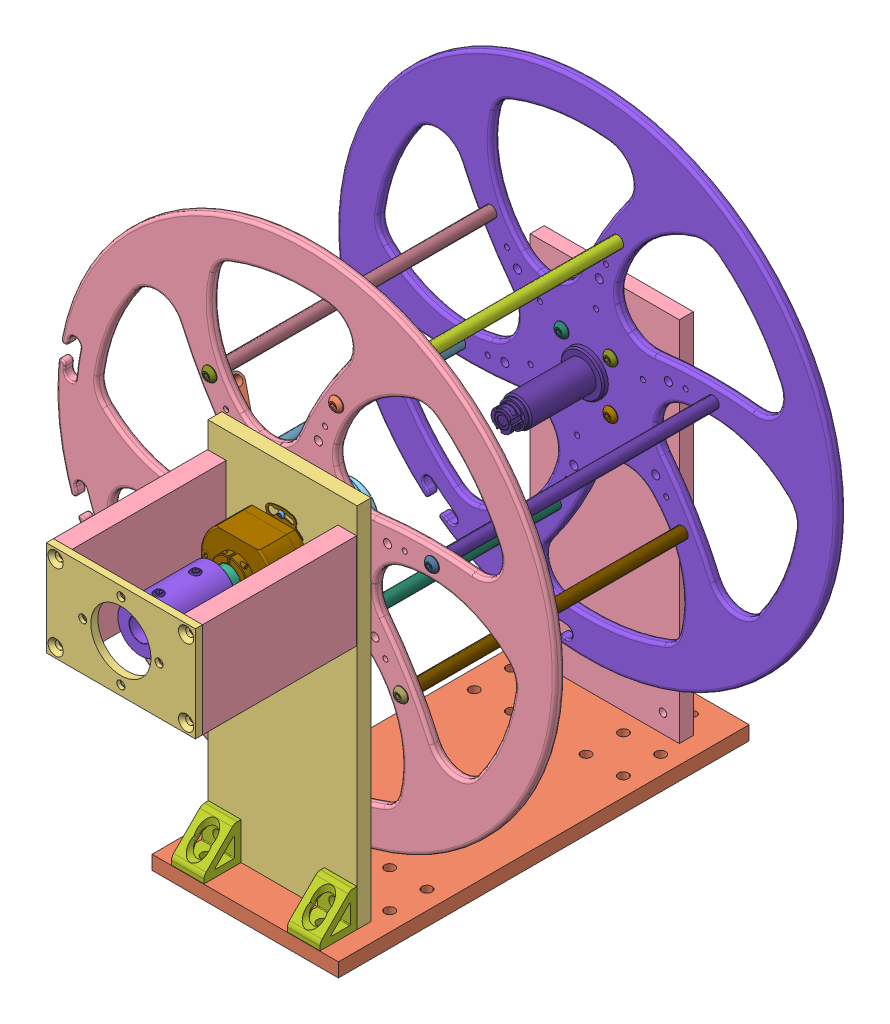
SolidWorks assembly MHK_PTO.step, configuration Default. Lengths in mm.
Overall size (340 379.53 364.56).
52 component instances, 45 part files, 0 mates.
Components (placement in the parent):
- Spool Support.step-1: Spool Support.step [Default] at (-13.1975 -9.525 242.4976) x (0 0 -1) z (1 0 0) size (279.85 259.52 127)
  - 92095A113.step-1: 92095A113.step [Default] at (-52.0594 229.525 13.1975) x (0 0 -1) z (-1 0 0) size (4.5 4.5 4.5)
  - 92095A113.step-2: 92095A113.step [Default] at (-52.0594 189.525 13.1975) x (0 0 -1) z (-1 0 0) size (4.5 4.5 4.5)
  - Spool Support-0.step-1: Spool Support-0.step [Default] at origin size (279.85 9.53 127)
  - Spool Support-1.step-1: Spool Support-1.step [Default] at origin size (9.52 250 101.6)
  - Spool Support-2.step-1: Spool Support-2.step [Default] at origin size (9.53 250 101.6)
- Spool Core.step-1: Spool Core.step [Default] at (13.4446 195.1511 -61.4824) x (0 1 0) z (0 0 1) size (370 340 273.99)
  - Component13.step-1: Component13.step [Default] at (-7.5076 6.2623 17.1) x (0.766044 -0.642788 0) z (0 0 1) size (9.5 9.5 14.75)
  - Component14.step-1: Component14.step [Default] at (-10.8225 46.1728 670.1648) x (1 0 0) z (0 0 -1) size (9.5 9.5 14.75)
  - 47065T663.step-1: 47065T663.step [Default] at (-195.1511 -26.1946 353.8432) x (0 0 1) z (0 1 0) size (25.4 25.4 22.23)
  - Spool Core-3.step-1: Spool Core-3.step [Default] at origin size (340 340 6.35)
  - Spool Core-4.step-1: Spool Core-4.step [Default] at origin size (9.5 9.5 14.75)
  - Spool Core-5.step-1: Spool Core-5.step [Default] at origin size (8.18 8.18 9.12)
  - Spool Core-6.step-1: Spool Core-6.step [Default] at origin size (9.5 9.5 14.75)
  - Spool Core-7.step-1: Spool Core-7.step [Default] at origin size (9.5 9.5 14.75)
  - Spool Core-8.step-1: Spool Core-8.step [Default] at origin size (8 8 185)
  - Spool Core-9.step-1: Spool Core-9.step [Default] at origin size (8 8 185)
  - Spool Core-10.step-1: Spool Core-10.step [Default] at origin size (8 8 185)
  - Spool Core-11.step-1: Spool Core-11.step [Default] at origin size (9.5 9.5 14.75)
  - Spool Core-12.step-1: Spool Core-12.step [Default] at origin size (8 8 185)
  - Spool Core-13.step-1: Spool Core-13.step [Default] at origin size (8 8 185)
  - Spool Core-14.step-1: Spool Core-14.step [Default] at origin size (9.5 9.5 14.75)
  - Spool Core-15.step-1: Spool Core-15.step [Default] at origin size (9.5 9.5 14.75)
  - Spool Core-16.step-1: Spool Core-16.step [Default] at origin size (9.5 9.5 14.75)
  - Spool Core-17.step-1: Spool Core-17.step [Default] at origin size (340 340 6.35)
  - Spool Core-18.step-1: Spool Core-18.step [Default] at origin size (17.75 23.28 7.94)
  - Spool Core-19.step-1: Spool Core-19.step [Default] at origin size (9.5 9.5 14.75)
  - Spool Core-20.step-1: Spool Core-20.step [Default] at origin size (8 8 185)
  - Spool Core-21.step-1: Spool Core-21.step [Default] at origin size (23.39 18.02 7.94)
  - Spool Core-22.step-1: Spool Core-22.step [Default] at origin size (9.5 9.5 14.75)
  - Spool Core-23.step-1: Spool Core-23.step [Default] at origin size (9.5 9.5 14.75)
  - Spool Core-24.step-1: Spool Core-24.step [Default] at origin size (9.5 9.5 14.75)
  - Spool Core-25.step-1: Spool Core-25.step [Default] at origin size (9.5 9.5 14.75)
  - Spool Core-26.step-1: Spool Core-26.step [Default] at origin size (8.18 8.18 9.12)
  - Spool Core-27.step-1: Spool Core-27.step [Default] at origin size (9.5 9.5 14.75)
  - Spool Core-28.step-1: Spool Core-28.step [Default] at origin size (9.5 9.5 14.75)
  - Spool Core-29.step-1: Spool Core-29.step [Default] at origin size (9.5 9.5 14.75)
  - Spool Core-30.step-1: Spool Core-30.step [Default] at origin size (56 56 99.65)
  - Spool Core-31.step-1: Spool Core-31.step [Default] at origin size (8.18 8.18 9.12)
  - Spool Core-32.step-1: Spool Core-32.step [Default] at origin size (9.5 9.5 14.75)
  - Spool Core-33.step-1: Spool Core-33.step [Default] at origin size (23.71 23.42 7.94)
- Motor Support.step-1: Motor Support.step [Default] at (-17.8977 208.142 442.889) x (0 0 1) z (-1 0 0) size (109.83 65 101.6)
  - Component1.step-1: Component1.step [Default] at (-45 0 0) size (4.83 65 101.6)
  - Component2.step-1: Component2.step [Default] at (-7.2906 1.3024 20.2023) size (105 65 12.7)
  - Component2.step-2: Component2.step [Default] at (-7.2906 1.3024 -68.6977) size (105 65 12.7)
- Shaft Clamp.step-1: Shaft Clamp.step [Default] at (0 200 264.925) x (0.707107 0.707107 0) z (0 0 1) size (63 63 21)
- Shaft.step-1: Shaft.step [Default] at (0 200 257.525) size (16 16 118.4)
- Shaft Clamp Adapter.step-1: Shaft Clamp Adapter.step [Default] at (0 200 270.425) x (0 0 -1) z (0.707107 0.707107 0) size (6.35 66.29 66.29)
- Shaft Coupler.step-1: Shaft Coupler.step [Default] at (0 200 364.525) size (31 31.76 50.01)
- Encoder.step-1: Encoder.step [Default] at (0 200 304.36) x (1 0 0) z (0 0 -1) size (50.8 52.34 36.53)
- 47065T663.step-1: 47065T663.step [Default] at (39.6392 0 292.3608) x (0 0 1) z (-1 0 0) size (25.4 25.4 22.23)
- 47065T663.step-2: 47065T663.step [Default] at (-39.3608 0 292.3608) x (0 0 1) z (-1 0 0) size (25.4 25.4 22.23)
